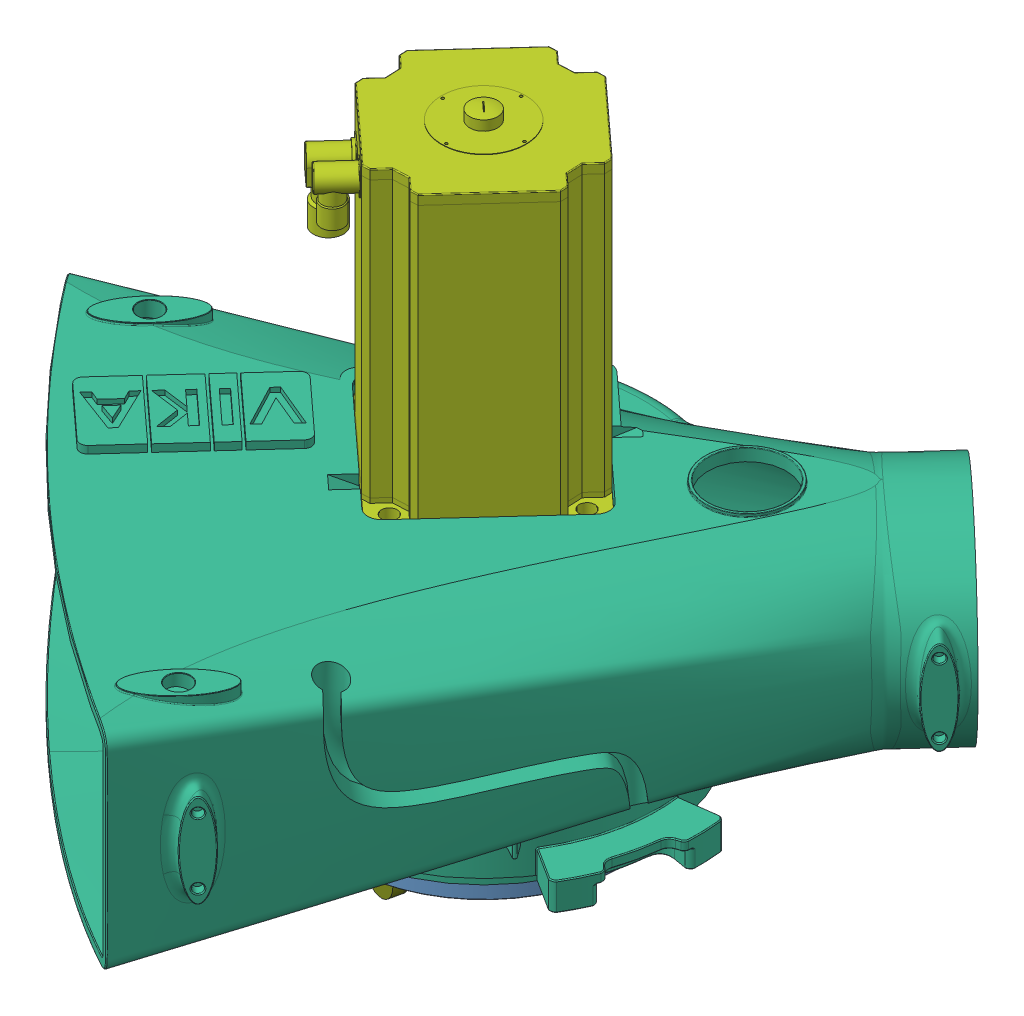
SolidWorks assembly GearBox3, configuration Default. Lengths in mm.
Overall size (948.21 720.15 952.05).
33 component instances, 25 part files, 73 mates.
Components (placement in the parent):
- SIR2-120_InternalRingGear(GearBox3)-1: SIR2-120_InternalRingGear(GearBox3) [Default] at origin size (300 20.1 300)
- RU_228(G)(GearBox3)-1: RU_228(G)(GearBox3) [Default] at (245.8223 27.5 -90.7039) x (0 -1 0) z (-0.999976 0 0.006943) size (35 302.08 302.08) (flexible)
  - RU_228(G)_Inner(GearBox3)-1: RU_228(G)_Inner(GearBox3) [Default] at (0 88.995 246.4461) x (1 0 0) z (0 0.222244 -0.974991) size (35 225.5 225.5)
  - RU_228(G)_Outer(GearBox3)-1: RU_228(G)_Outer(GearBox3) [Default] at (0 88.995 246.4461) x (1 0 0) z (0 -0.006943 0.999976) size (35 300 300)
  - RU_228G_Roller(GearBox3)-1: RU_228G_Roller(GearBox3) [Default] at (0 196.9114 282.4061) size (15.9 15.9 15.9)
- SKF_6021-1: SKF_6021 [Default] at (0 23 0) x (0 -1 0) z (0.799482 0 -0.60069) size (26.17 163.17 163.17)
- Body3-1: Body3 [Default] at (244.7299 195 -178.7014) x (0 -1 0) z (-0.674857 0 0.737948) size (316.2 642.13 702.9)
- Servo_Axis_1-2-3-1: Servo_Axis_1-2-3 [Default] at (-0.098 607.5 0.0044) x (-0.738573 0 -0.674174) z (-0.674174 0 0.738573) size (190 412 229) (flexible)
  - AEG-69-225-468_6,6kW_21-Nm-1: AEG-69-225-468_6,6kW_21-Nm [Default] at origin size (190 342 229)
  - ServoShaft_30mm-1: ServoShaft_30mm [Default] at (0 69 0) x (0.061016 0 -0.998137) z (0.998137 0 0.061016) size (30 330 30)
  - SKF_16006-1: SKF_16006 [Default] at (0 320.5 0) x (0 1 0) z (-0.978278 0 0.207296) size (9 55 55)
- Axis3_GearBoxFixedPart-1: Axis3_GearBoxFixedPart [Default] at (0 405.1351 0) x (0 1 0) z (0.21547 0 -0.976511) size (110 220 220)
- Gearbox3_ServoShaft-1: Gearbox3_ServoShaft [Default] at (0 24 0) x (0.269483 0 -0.963005) z (0.963005 0 0.269483) size (36.5 245 36.5)
- SKF_61804-1: SKF_61804 [Default] at (0 27.5 0) x (0 -1 0) z (0 0 1) size (7.11 32.85 32.78)
- SKF_61804-2: SKF_61804 [Default] at (0 110.5 0) x (0 -1 0) z (0 0 1) size (7.11 32.85 32.78)
- SKF_61804-3: SKF_61804 [Default] at (8.1878 88.5 -37.1074) x (0 1 0) z (0 0 1) size (7.11 32.85 32.78)
- GearBox3_BevelShaft-1: GearBox3_BevelShaft [Default] at (8.1878 -38 -37.1074) x (-0.97892 0 0.204246) z (0 -1 0) size (20 20 130)
- SSA1-32(GearBox3)-1: SSA1-32(GearBox3) [Default] at (8.1878 62 -37.1074) x (-0.97892 0 0.204246) z (0 -1 0) size (52 52 15.1)
- mmsa2-20R_BevelGear(GearBox2)-1: mmsa2-20R_BevelGear(GearBox2) [Default] at (8.1878 -20 -37.1074) x (-0.97892 0 0.204246) z (0.204246 0 0.97892) size (54.75 25.25 51.87)
- SKF_61804-5: SKF_61804 [Default] at (8.1878 6.5 -37.1074) x (0 -1 0) z (0.004387 0 0.99999) size (7.11 32.85 32.78)
- BevelGear_Keeper(GearBox3)-1: BevelGear_Keeper(GearBox3) [Default] at (0 2.5 0) x (0.21547 0 -0.976511) z (0 -1 0) size (195 195 83)
- mmsa2-20L_BevelGear(GearBox2)-1: mmsa2-20L_BevelGear(GearBox2) [Default] at (16.0525 -56 -72.75) x (0.864262 -0.465494 0.190702) z (-0.45456 -0.885051 -0.1003) size (54.26 25.25 51.03)
- BevelShaft(GearBox3)-1: BevelShaft(GearBox3) [Default] at (-20.3619 -56 92.2802) x (-0.864262 0.465494 -0.190702) z (-0.45456 -0.885051 -0.1003) size (15 189 15)
- SKF_61902-1: SKF_61902 [Default] at (-17.884 -56 81.0504) x (0.21547 0 -0.976511) z (0.976511 0 0.21547) size (7.1 28.75 28.69)
- SKF_61902-2: SKF_61902 [Default] at (17.884 -56 -81.0504) x (0.21547 0 -0.976511) z (0.976511 0 0.21547) size (7.1 28.75 28.69)
- KWGDL2-R1_WormGear(Gearbox2)-1: KWGDL2-R1_WormGear(Gearbox2) [Default] at (2.047 -56 -9.2769) x (-0.864262 0.465494 -0.190702) z (0.45456 0.885051 0.1003) size (38.22 84 44.07)
- WormWheelShaft(GearBox3)-1: WormWheelShaft(GearBox3) [Default] at (-57.6598 -99.65 29.2635) x (0.987358 0 0.158503) z (-0.158503 0 0.987358) size (30 103 30)
- SKF_61902-3: SKF_61902 [Default] at (-57.6598 3.5 29.2635) x (0 1 0) z (0 0 1) size (7.1 28.75 28.69)
- AGDL2_WormWheel(GearBox3)-1: AGDL2_WormWheel(GearBox3) [Default] at (-57.6598 -63.5 29.2635) x (0 -1 0) z (-0.987358 0 -0.158503) size (37.7 70.95 71.04)
- SSA2_5-42(GearBox3)-1: SSA2_5-42(GearBox3) [Default] at (51.5654 -9.5 35.4845) x (0.968834 0 0.24771) z (-0.24771 0 0.968834) size (130 15.1 129.89)
- SSA2-52(GearBox3)-1: SSA2-52(GearBox3) [Default] at (-57.6598 -15.15 29.2635) x (0.987358 0 0.158503) z (-0.158503 0 0.987358) size (94 15.1 93.86)
- SKF_61902-4: SKF_61902 [Default] at (51.5654 1.5 35.4845) x (0 1 0) z (0.087906 0 0.996129) size (7.1 28.75 28.69)
- SpurShaft(GearBox3)-1: SpurShaft(GearBox3) [Default] at (51.5654 5 35.4845) x (-0.968834 0 -0.24771) z (-0.24771 0 0.968834) size (30 55 30)
Mates (geometry in assembly coordinates):
- Coincident1: coincident anti-aligned: line of SIR2-120_InternalRingGear(GearBox3)-1 through (51.6327 0 0) axis (0 0 1); line of RU_228(G)(GearBox3)-1/RU_228(G)_Outer(GearBox3)-1 through (33 0 44) axis (0 0 -1)
- Concentric2: concentric aligned: cylinder of SIR2-120_InternalRingGear(GearBox3)-1 through (-107.2462 -10.05 -89.9903) axis (0 1 0) radius 5; cylinder of RU_228(G)(GearBox3)-1/RU_228(G)_Outer(GearBox3)-1 through (-107.2462 45 -89.9903) axis (0 1 0) radius 8
- Concentric3: concentric aligned: cylinder of SIR2-120_InternalRingGear(GearBox3)-1 through (107.2462 -10.05 89.9903) axis (0 1 0) radius 5; cylinder of RU_228(G)(GearBox3)-1/RU_228(G)_Outer(GearBox3)-1 through (107.2462 45 89.9903) axis (0 1 0) radius 8
- Coincident2: coincident anti-aligned: plane of SIR2-120_InternalRingGear(GearBox3)-1 through (0 10 0) normal (0 1 0); plane of RU_228(G)(GearBox3)-1/RU_228(G)_Outer(GearBox3)-1 through (0 10 0) normal (0 -1 0)
- Coincident3: coincident aligned: plane of SIR2-120_InternalRingGear(GearBox3)-1 through (0 0 0) normal (0 1 0); plane of assembly through (0 0 0) normal (0 1 0)
- Coincident4: coincident aligned: plane of SIR2-120_InternalRingGear(GearBox3)-1 through (0 0 0) normal (1 0 0); plane of assembly through (0 0 0) normal (1 0 0)
- Coincident5: coincident aligned: plane of SIR2-120_InternalRingGear(GearBox3)-1 through (0 0 0) normal (0 0 1); plane of assembly through (0 0 0) normal (0 0 1)
- Coincident8: coincident anti-aligned: line of SIR2-120_InternalRingGear(GearBox3)-1 through (51.6327 0 0) axis (0 0 1); line of SKF_6021-1 through (26 0 36) axis (0 0 -1)
- Coincident9: coincident aligned: plane of RU_228(G)(GearBox3)-1/RU_228(G)_Inner(GearBox3)-1 through (0 10 0) normal (0 -1 0); plane of SKF_6021-1 through (0 10 0) normal (0 -1 0)
- Coincident10: coincident aligned: line of SIR2-120_InternalRingGear(GearBox3)-1 through (51.6327 0 0) axis (0 0 1); line of Body3-1 through (0 272.5 0) axis (0 1 0)
- Concentric4: concentric aligned: cylinder of RU_228(G)(GearBox3)-1/RU_228(G)_Inner(GearBox3)-1 through (68.2602 10 62.4243) axis (0 -1 0) radius 5.25; cylinder of Body3-1 through (68.2602 331.2014 62.4243) axis (0 -1 0) radius 5.25
- Coincident11: coincident anti-aligned: plane of RU_228(G)(GearBox3)-1/RU_228(G)_Inner(GearBox3)-1 through (0 45 0) normal (0 1 0); plane of Body3-1 through (114.382 45 104.6029) normal (0 -1 0)
- Concentric6: concentric anti-aligned: cylinder of Body3-1 through (105.7921 58.6711 -4.8225) axis (0 1 0) radius 8.5; cylinder of Servo_Axis_1-2-3-1/AEG-69-225-468_6,6kW_21-Nm-1 through (105.7921 607.501 -4.8225) axis (0 -1 0) radius 8.5
- Concentric7: concentric anti-aligned: cylinder of Body3-1 through (-105.9881 58.6711 4.8313) axis (0 1 0) radius 8.5; cylinder of Servo_Axis_1-2-3-1/AEG-69-225-468_6,6kW_21-Nm-1 through (-105.988 607.501 4.8313) axis (0 -1 0) radius 8.5
- Coincident12: coincident anti-aligned: plane of Body3-1 through (-5.1103 282.5 -114.4373) normal (0 1 0); plane of Servo_Axis_1-2-3-1/AEG-69-225-468_6,6kW_21-Nm-1 through (-0.098 282.5 0.0044) normal (0 -1 0)
- Coincident13: coincident anti-aligned: line of SIR2-120_InternalRingGear(GearBox3)-1 through (51.6327 0 0) axis (0 0 1); line of Axis3_GearBoxFixedPart-1 through (35 0 115) axis (0 0 -1)
- Coincident14: coincident anti-aligned: plane of Body3-1 through (114.382 55 104.6029) normal (0 1 0); plane of Axis3_GearBoxFixedPart-1 through (107.4162 55 23.7017) normal (0 -1 0)
- Concentric8: concentric anti-aligned: cylinder of Body3-1 through (-19.9309 331.2014 90.3272) axis (0 -1 0) radius 5.25; cylinder of Axis3_GearBoxFixedPart-1 through (-19.9309 4.999 90.3272) axis (0 1 0) radius 5.25
- Coincident15: coincident anti-aligned: line of Axis3_GearBoxFixedPart-1 through (35 0 115) axis (0 0 -1); line of Gearbox3_ServoShaft-1 through (90 0 179) axis (0 0 1)
- Coincident19: coincident anti-aligned: plane of Axis3_GearBoxFixedPart-1 through (15.6242 24 3.4475) normal (0 1 0); plane of Gearbox3_ServoShaft-1 through (0 24 0) normal (0 -1 0)
- Concentric12: concentric anti-aligned: cylinder of Gearbox3_ServoShaft-1 through (0 179 0) axis (0 1 0) radius 10; cylinder of SKF_61804-1 through (0 27.5 0) axis (0 -1 0) radius 10
- Coincident21: coincident anti-aligned: plane of Axis3_GearBoxFixedPart-1 through (15.6242 24 3.4475) normal (0 1 0); plane of SKF_61804-1 through (0 24 0) normal (0 -1 0)
- Concentric14: concentric anti-aligned: cylinder of Axis3_GearBoxFixedPart-1 through (0 114 0) axis (0 1 0) radius 16; cylinder of SKF_61804-2 through (0 110.5 0) axis (0 -1 0) radius 16
- Coincident22: coincident anti-aligned: plane of Axis3_GearBoxFixedPart-1 through (15.6242 107 3.4475) normal (0 1 0); plane of SKF_61804-2 through (0 107 0) normal (0 -1 0)
- Concentric16: concentric anti-aligned: cylinder of Axis3_GearBoxFixedPart-1 through (8.1878 5 -37.1074) axis (0 -1 0) radius 16; cylinder of SKF_61804-3 through (8.1878 88.5 -37.1074) axis (0 1 0) radius 16
- Coincident24: coincident anti-aligned: plane of Axis3_GearBoxFixedPart-1 through (23.812 92 -33.6599) normal (0 -1 0); plane of SKF_61804-3 through (8.1878 92 -37.1074) normal (0 1 0)
- Concentric17: concentric aligned: cylinder of GearBox3_BevelShaft-1 through (8.1878 92 -37.1074) axis (0 1 0) radius 10; cylinder of SSA1-32(GearBox3)-1 through (8.1878 54.5 -37.1074) axis (0 1 0) radius 10
- Coincident25: coincident aligned: plane of GearBox3_BevelShaft-1 through (4.2227 54.5 -48.1554) normal (0.97892 0 -0.204246); plane of SSA1-32(GearBox3)-1 through (4.2227 54.45 -48.1554) normal (0.97892 0 -0.204246)
- Coincident26: coincident anti-aligned: plane of GearBox3_BevelShaft-1 through (8.1878 69.5 -37.1074) normal (0 -1 0); plane of SSA1-32(GearBox3)-1 through (8.1878 69.5 -37.1074) normal (0 1 0)
- Coincident28: coincident anti-aligned: plane of Axis3_GearBoxFixedPart-1 through (23.812 92 -33.6599) normal (0 -1 0); plane of GearBox3_BevelShaft-1 through (-1.6014 92 -35.0649) normal (0 1 0)
- GearMate1: gear = 32 : 18 mm: cylinder of Gearbox3_ServoShaft-1 through (0 74 0) axis (0 -1 0) radius 15; cylinder of SSA1-32(GearBox3)-1 through (8.1878 54.5 -37.1074) axis (0 1 0) radius 26
- Parallel5: parallel aligned: plane of GearBox3_BevelShaft-1 through (4.9376 -23 -44.7292) normal (0.97892 0 -0.204246); plane of mmsa2-20R_BevelGear(GearBox2)-1 through (4.8813 -20 -45.6113) normal (0.97892 0 -0.204246)
- Coincident35: coincident aligned: line of GearBox3_BevelShaft-1 through (8.1878 -3 -37.1074) axis (0 1 0); line of mmsa2-20R_BevelGear(GearBox2)-1 through (8.1878 -28 -37.1074) axis (0 1 0)
- Coincident36: coincident aligned: plane of GearBox3_BevelShaft-1 through (0.8459 -38 -35.5756) normal (0 -1 0); plane of mmsa2-20R_BevelGear(GearBox2)-1 through (8.1878 -38 -37.1074) normal (0 -1 0)
- Concentric18: concentric anti-aligned: cylinder of GearBox3_BevelShaft-1 through (8.1878 92 -37.1074) axis (0 1 0) radius 7.5; cylinder of SKF_61804-5 through (8.1878 6.5 -37.1074) axis (0 -1 0) radius 10
- Coincident37: coincident anti-aligned: plane of Axis3_GearBoxFixedPart-1 through (23.812 10 -33.6599) normal (0 -1 0); plane of SKF_61804-5 through (8.1878 10 -37.1074) normal (0 1 0)
- Concentric19: concentric aligned: cylinder of Axis3_GearBoxFixedPart-1 through (8.1878 5 -37.1074) axis (0 -1 0) radius 16; cylinder of SKF_61804-5 through (8.1878 6.5 -37.1074) axis (0 -1 0) radius 16
- Concentric20: concentric anti-aligned: cylinder of SKF_61804-5 through (8.1878 6.5 -37.1074) axis (0 -1 0) radius 16; cylinder of BevelGear_Keeper(GearBox3)-1 through (8.1878 0 -37.1074) axis (0 1 0) radius 16
- Concentric21: concentric aligned: cylinder of Axis3_GearBoxFixedPart-1 through (29.2953 15 6.4641) axis (0 -1 0) radius 5; cylinder of BevelGear_Keeper(GearBox3)-1 through (29.2953 5 6.4641) axis (0 -1 0) radius 5
- Coincident38: coincident anti-aligned: plane of Axis3_GearBoxFixedPart-1 through (51.2668 5 11.3122) normal (0 -1 0); plane of BevelGear_Keeper(GearBox3)-1 through (0 5 0) normal (0 1 0)
- Concentric22: concentric aligned: cylinder of BevelGear_Keeper(GearBox3)-1 through (17.1298 -56 -77.6326) axis (0.21547 0 -0.976511) radius 8.5; cylinder of mmsa2-20L_BevelGear(GearBox2)-1 through (16.0525 -56 -72.75) axis (0.21547 0 -0.976511) radius 7.5
- GearMate2: gear = 35 : 35 mm: circle of mmsa2-20R_BevelGear(GearBox2)-1; circle of mmsa2-20L_BevelGear(GearBox2)-1
- Concentric23: concentric aligned: cylinder of BevelGear_Keeper(GearBox3)-1 through (17.1298 -56 -77.6326) axis (0.21547 0 -0.976511) radius 8.5; cylinder of BevelShaft(GearBox3)-1 through (20.3619 -56 -92.2802) axis (0.21547 0 -0.976511) radius 7.5
- Coincident39: coincident aligned: plane of BevelGear_Keeper(GearBox3)-1 through (20.3619 2.5 -92.2802) normal (0.21547 0 -0.976511); plane of BevelShaft(GearBox3)-1 through (13.8799 -52.5088 -93.7105) normal (0.21547 0 -0.976511)
- Coincident40: coincident anti-aligned: plane of mmsa2-20L_BevelGear(GearBox2)-1 through (16.0525 -56 -72.75) normal (0.21547 0 -0.976511); plane of BevelShaft(GearBox3)-1 through (16.0525 -56 -72.75) normal (-0.21547 0 0.976511)
- Coincident41: coincident aligned: plane of mmsa2-20L_BevelGear(GearBox2)-1 through (21.4399 -48.7328 -71.5613) normal (-0.864262 0.465494 -0.190702); plane of BevelShaft(GearBox3)-1 through (17.5615 -48.7328 -53.9841) normal (-0.864262 0.465494 -0.190702)
- Concentric24: concentric anti-aligned: cylinder of BevelGear_Keeper(GearBox3)-1 through (18.6381 -56 -84.4682) axis (-0.21547 0 0.976511) radius 14; cylinder of SKF_61902-2 through (17.884 -56 -81.0504) axis (0.21547 0 -0.976511) radius 14
- Coincident42: coincident anti-aligned: plane of BevelGear_Keeper(GearBox3)-1 through (18.6381 -56 -84.4682) normal (-0.21547 0 0.976511); plane of SKF_61902-2 through (18.6381 -56 -84.4682) normal (0.21547 0 -0.976511)
- Concentric25: concentric aligned: cylinder of BevelGear_Keeper(GearBox3)-1 through (-18.6381 -56 84.4682) axis (0.21547 0 -0.976511) radius 14; cylinder of SKF_61902-1 through (-17.884 -56 81.0504) axis (0.21547 0 -0.976511) radius 14
- Coincident43: coincident anti-aligned: plane of BevelGear_Keeper(GearBox3)-1 through (-18.6381 -56 84.4682) normal (0.21547 0 -0.976511); plane of SKF_61902-1 through (-18.6381 -56 84.4682) normal (-0.21547 0 0.976511)
- Coincident44: coincident aligned: line of SKF_61902-1 through (-18.6381 -56 84.4682) axis (0.21547 0 -0.976511); line of KWGDL2-R1_WormGear(Gearbox2)-1 through (-16.0525 -56 72.75) axis (0.21547 0 -0.976511)
- Coincident45: coincident anti-aligned: plane of BevelShaft(GearBox3)-1 through (2.047 -56 -9.2769) normal (-0.21547 0 0.976511); plane of KWGDL2-R1_WormGear(Gearbox2)-1 through (2.047 -56 -9.2769) normal (0.21547 0 -0.976511)
- Coincident46: coincident aligned: plane of BevelShaft(GearBox3)-1 through (1.6096 -47.3363 5.9875) normal (0.864262 -0.465494 0.190702); plane of KWGDL2-R1_WormGear(Gearbox2)-1 through (0.6954 -47.3363 10.1304) normal (0.864262 -0.465494 0.190702)
- Concentric27: concentric anti-aligned: cylinder of BevelGear_Keeper(GearBox3)-1 through (-57.6598 7.001 29.2635) axis (0 -1 0) radius 14; line of SKF_61902-3 through (-57.6598 0 29.2635) axis (0 1 0)
- Coincident49: coincident aligned: plane of BevelGear_Keeper(GearBox3)-1 through (0 0 0) normal (0 -1 0); plane of SKF_61902-3 through (-57.6598 0 29.2635) normal (0 -1 0)
- Concentric28: concentric aligned: cylinder of WormWheelShaft(GearBox3)-1 through (-57.6598 3.35 29.2635) axis (0 1 0) radius 7.5; line of SKF_61902-3 through (-57.6598 0 29.2635) axis (0 1 0)
- Concentric31: concentric aligned: cylinder of WormWheelShaft(GearBox3)-1 through (-57.6598 3.35 29.2635) axis (0 1 0) radius 10; cylinder of AGDL2_WormWheel(GearBox3)-1 through (-57.6598 -63.5 29.2635) axis (0 1 0) radius 10
- Coincident51: coincident anti-aligned: plane of WormWheelShaft(GearBox3)-1 through (-47.7862 -44.65 30.8485) normal (0 -1 0); plane of AGDL2_WormWheel(GearBox3)-1 through (-59.2448 -44.65 39.137) normal (0 1 0)
- Coincident52: coincident aligned: plane of WormWheelShaft(GearBox3)-1 through (-61.1068 -40.0538 40.4839) normal (0.987358 0 0.158503); plane of AGDL2_WormWheel(GearBox3)-1 through (-61.1068 -44.65 40.4839) normal (0.987358 0 0.158503)
- GearMate4: gear = 30 : 25 mm: cylinder of KWGDL2-R1_WormGear(Gearbox2)-1 through (2.047 -56 -9.2769) axis (0.21547 0 -0.976511) radius 12.5; cylinder of AGDL2_WormWheel(GearBox3)-1 through (-57.6598 -63.5 29.2635) axis (0 1 0) radius 15
- Distance1: distance = 22.65 mm anti-aligned: plane of BevelGear_Keeper(GearBox3)-1 through (0 0 0) normal (0 -1 0); plane of WormWheelShaft(GearBox3)-1 through (-42.8494 -22.65 31.641) normal (0 1 0)
- Concentric32: concentric anti-aligned: cylinder of BevelGear_Keeper(GearBox3)-1 through (51.5654 7 35.4845) axis (0 -1 0) radius 14; cylinder of SSA2_5-42(GearBox3)-1 through (51.5654 -17.05 35.4845) axis (0 1 0) radius 9.25
- Concentric33: concentric aligned: cylinder of WormWheelShaft(GearBox3)-1 through (-57.6598 3.35 29.2635) axis (0 1 0) radius 9; cylinder of SSA2-52(GearBox3)-1 through (-57.6598 -22.7003 29.2635) axis (0 1 0) radius 9
- Coincident53: coincident aligned: plane of WormWheelShaft(GearBox3)-1 through (-54.3712 -27.2462 19.0303) normal (-0.987358 0 -0.158503); plane of SSA2-52(GearBox3)-1 through (-56.0553 -22.7003 29.521) normal (-0.987358 0 -0.158503)
- Coincident54: coincident anti-aligned: circle of WormWheelShaft(GearBox3)-1; plane of SSA2-52(GearBox3)-1 through (-57.6598 -22.65 29.2635) normal (0 -1 0)
- Concentric34: concentric anti-aligned: cylinder of BevelGear_Keeper(GearBox3)-1 through (51.5654 7 35.4845) axis (0 -1 0) radius 14; cylinder of SKF_61902-4 through (51.5654 1.5 35.4845) axis (0 1 0) radius 14
- Coincident55: coincident anti-aligned: circle of BevelGear_Keeper(GearBox3)-1; plane of SKF_61902-4 through (51.5654 5 35.4845) normal (0 1 0)
- Coincident57: coincident aligned: plane of SKF_61902-4 through (51.5654 5 35.4845) normal (0 1 0); plane of SpurShaft(GearBox3)-1 through (44.2992 5 33.6266) normal (0 1 0)
- Coincident58: coincident aligned: line of SKF_61902-4 through (51.5654 -2 35.4845) axis (0 1 0); line of SpurShaft(GearBox3)-1 through (51.5654 -27 35.4845) axis (0 1 0)
- Coincident59: coincident aligned: plane of SSA2_5-42(GearBox3)-1 through (53.1398 -17.05 35.887) normal (-0.968834 0 -0.24771); plane of SpurShaft(GearBox3)-1 through (50.5079 -21.5962 46.1808) normal (-0.968834 0 -0.24771)
- Coincident60: coincident anti-aligned: plane of SSA2_5-42(GearBox3)-1 through (51.5654 -17 35.4845) normal (0 -1 0); plane of SpurShaft(GearBox3)-1 through (42.8459 -17 33.2551) normal (0 1 0)
- GearMate5: gear = 120 : 58 mm: circle of SSA2_5-42(GearBox3)-1; circle of SIR2-120_InternalRingGear(GearBox3)-1
- GearMate6: gear = 58 : 42 mm: circle of SSA2-52(GearBox3)-1; circle of SSA2_5-42(GearBox3)-1
